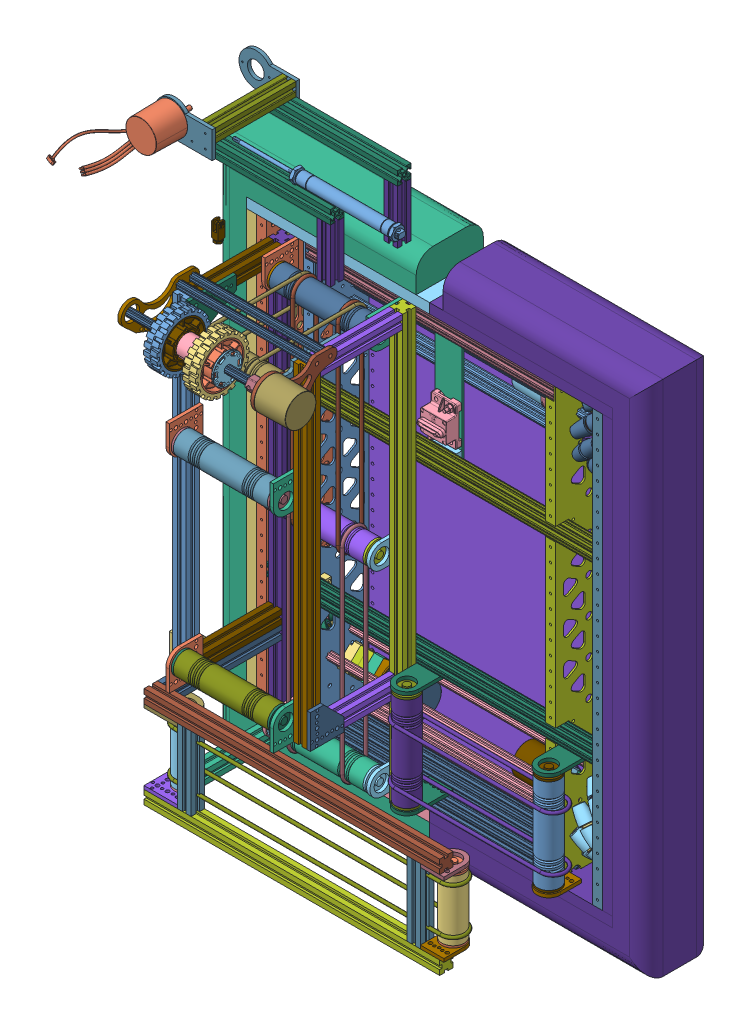
SolidWorks assembly Robot 2020, configuration Default. Lengths in mm. (continued)
Components (placement in the parent): (continued)
- Robot 2020(2)^Robot 2020-1: Robot 2020(2)^Robot 2020 [Default] at origin size (819.15 992.53 549) (virtual) (continued)
  - Fame 2020^Robot 2020(2)_Robot 2020-1: Fame 2020^Robot 2020(2)_Robot 2020 [Default] at origin size (819.15 977.9 171.99) (virtual) (continued)
    - Left Wheel Assembly^Fame 2020_Robot 2020(2)_Robot 2020-1: Left Wheel Assembly^Fame 2020_Robot 2020(2)_Robot 2020 [Default] at (500 0 0) size (65.82 166.11 165.01) (virtual) (continued)
      - 6_Mecanum_Wheel_Left_217-2799^Left Wheel Assembly_Fame 2020_Robot 2020(2)_Robot 2020-1: 6_Mecanum_Wheel_Left_217-2799^Left Wheel Assembly_Fame 2020_Robot 2020(2)_Robot 2020 [Default] x (0 0 1) z (-1 0 0) size (165.01 166.11 65.82) (virtual) (continued)
        - 217-2586-005 Rev2^6_Mecanum_Wheel_Left_217-2799_Left Wheel Assembly_Fame 2020_Robot 2020(2)_Robot 2020-9: 217-2586-005 Rev2^6_Mecanum_Wheel_Left_217-2799_Left Wheel Assembly_Fame 2020_Robot 2020(2)_Robot 2020 [Default] at (85.9856 -351.4028 221.3312) x (-0.32102 -0.630037 -0.707107) z (-0.857032 -0.124484 0.5) size (8.5 8 8) (virtual)
        - 217-2586-005 Rev2^6_Mecanum_Wheel_Left_217-2799_Left Wheel Assembly_Fame 2020_Robot 2020(2)_Robot 2020-10: 217-2586-005 Rev2^6_Mecanum_Wheel_Left_217-2799_Left Wheel Assembly_Fame 2020_Robot 2020(2)_Robot 2020 [Default] at (56.0127 -375.8444 221.3312) x (-0.630037 -0.32102 -0.707107) z (-0.766523 0.403042 0.5) size (8.5 8 8) (virtual)
        - 217-2586-005 Rev2^6_Mecanum_Wheel_Left_217-2799_Left Wheel Assembly_Fame 2020_Robot 2020(2)_Robot 2020-11: 217-2586-005 Rev2^6_Mecanum_Wheel_Left_217-2799_Left Wheel Assembly_Fame 2020_Robot 2020(2)_Robot 2020 [Default] at (17.3977 -378.0003 221.3312) x (-0.698401 0.110616 -0.707107) z (-0.383228 0.776618 0.5) size (8.5 8 8) (virtual)
        - 217-2586-005 Rev2^6_Mecanum_Wheel_Left_217-2799_Left Wheel Assembly_Fame 2020_Robot 2020(2)_Robot 2020-12: 217-2586-005 Rev2^6_Mecanum_Wheel_Left_217-2799_Left Wheel Assembly_Fame 2020_Robot 2020(2)_Robot 2020 [Default] at (-27.1128 -333.4898 233.9884) x (-0.110616 0.698401 -0.707107) z (0.620184 0.60446 0.5) size (8.5 8 8) (virtual)
        - 217-2586-005 Rev2^6_Mecanum_Wheel_Left_217-2799_Left Wheel Assembly_Fame 2020_Robot 2020(2)_Robot 2020-13: 217-2586-005 Rev2^6_Mecanum_Wheel_Left_217-2799_Left Wheel Assembly_Fame 2020_Robot 2020(2)_Robot 2020 [Default] at (-24.9569 -294.8748 233.9884) x (0.32102 0.630037 -0.707107) z (0.857032 0.124484 0.5) size (8.5 8 8) (virtual)
        - 217-2586-005 Rev2^6_Mecanum_Wheel_Left_217-2799_Left Wheel Assembly_Fame 2020_Robot 2020(2)_Robot 2020-14: 217-2586-005 Rev2^6_Mecanum_Wheel_Left_217-2799_Left Wheel Assembly_Fame 2020_Robot 2020(2)_Robot 2020 [Default] at (-0.5153 -264.9019 233.9884) x (0.630037 0.32102 -0.707107) z (0.766523 -0.403042 0.5) size (8.5 8 8) (virtual)
        - 217-2586-005 Rev2^6_Mecanum_Wheel_Left_217-2799_Left Wheel Assembly_Fame 2020_Robot 2020(2)_Robot 2020-15: 217-2586-005 Rev2^6_Mecanum_Wheel_Left_217-2799_Left Wheel Assembly_Fame 2020_Robot 2020(2)_Robot 2020 [Default] at (36.8759 -255.0196 233.9884) x (0.698401 -0.110616 -0.707107) z (0.383228 -0.776618 0.5) size (8.5 8 8) (virtual)
        - 217-2586-005 Rev2^6_Mecanum_Wheel_Left_217-2799_Left Wheel Assembly_Fame 2020_Robot 2020(2)_Robot 2020-16: 217-2586-005 Rev2^6_Mecanum_Wheel_Left_217-2799_Left Wheel Assembly_Fame 2020_Robot 2020(2)_Robot 2020 [Default] at (72.9347 -269.0028 233.9884) x (0.5 -0.5 -0.707107) z (-0.146447 -0.853553 0.5) size (8.5 8 8) (virtual)
        - 217-2586-005 Rev2^6_Mecanum_Wheel_Left_217-2799_Left Wheel Assembly_Fame 2020_Robot 2020(2)_Robot 2020-17: 217-2586-005 Rev2^6_Mecanum_Wheel_Left_217-2799_Left Wheel Assembly_Fame 2020_Robot 2020(2)_Robot 2020 [Default] at (93.8878 -301.5102 233.9884) x (0.110616 -0.698401 -0.707107) z (-0.620184 -0.60446 0.5) size (8.5 8 8) (virtual)
        - 217-2586-005 Rev2^6_Mecanum_Wheel_Left_217-2799_Left Wheel Assembly_Fame 2020_Robot 2020(2)_Robot 2020-18: 217-2586-005 Rev2^6_Mecanum_Wheel_Left_217-2799_Left Wheel Assembly_Fame 2020_Robot 2020(2)_Robot 2020 [Default] at (91.7319 -340.1252 233.9884) x (-0.32102 -0.630037 -0.707107) z (-0.857032 -0.124484 0.5) size (8.5 8 8) (virtual)
        - 217-2586-005 Rev2^6_Mecanum_Wheel_Left_217-2799_Left Wheel Assembly_Fame 2020_Robot 2020(2)_Robot 2020-19: 217-2586-005 Rev2^6_Mecanum_Wheel_Left_217-2799_Left Wheel Assembly_Fame 2020_Robot 2020(2)_Robot 2020 [Default] at (67.2903 -370.0981 233.9884) x (-0.630037 -0.32102 -0.707107) z (-0.766523 0.403042 0.5) size (8.5 8 8) (virtual)
        - 217-2586-005 Rev2^6_Mecanum_Wheel_Left_217-2799_Left Wheel Assembly_Fame 2020_Robot 2020(2)_Robot 2020-20: 217-2586-005 Rev2^6_Mecanum_Wheel_Left_217-2799_Left Wheel Assembly_Fame 2020_Robot 2020(2)_Robot 2020 [Default] at (29.8991 -379.9804 233.9884) x (-0.698401 0.110616 -0.707107) z (-0.383228 0.776618 0.5) size (8.5 8 8) (virtual)
      - 1_2_Hex_Bore_Aluminum_VersaHub_217-2592^Left Wheel Assembly_Fame 2020_Robot 2020(2)_Robot 2020-1: 1_2_Hex_Bore_Aluminum_VersaHub_217-2592^Left Wheel Assembly_Fame 2020_Robot 2020(2)_Robot 2020 [Default] at (-239.7248 -317.5 33.3875) x (-1 0 0) z (0 0.707107 0.707107) size (12.7 55.88 55.88) (virtual)
    - NEO Gearbox 2-stage Custom v5(Mirror) (2)^Fame 2020_Robot 2020(2)_Robot 2020-1: NEO Gearbox 2-stage Custom v5(Mirror) (2)^Fame 2020_Robot 2020(2)_Robot 2020 [Default] at (0 0 425) x (1 0 0) z (0 0 -1) size (164.9 90.53 90.53) (virtual)
      - VersaPlanetary_4_1_Gear_Kit_217-2818 v1(Mirror) (2)^NEO Gearbox 2-stage Custom v5(Mirror) (2)_Fame 2020_Robot 2020(2)_Robot 2020-1: VersaPlanetary_4_1_Gear_Kit_217-2818 v1(Mirror) (2)^NEO Gearbox 2-stage Custom v5(Mirror) (2)_Fame 2020_Robot 2020(2)_Robot 2020 [Default] at (-15.25 22.225 0) x (0 -0.707107 -0.707107) z (1 0 0) size (35.49 35.49 17.4) (virtual)
        - 217-2725-001 Rev1_24t Sun(Mirror) (2)^VersaPlanetary_4_1_Gear_Kit_217-2818 v1(Mirror) (2)_NEO Gearbox 2-stage Custom v5(Mirror) (2)_Fame 2020_Robot 2020(2)_Robot 2020-1: 217-2725-001 Rev1_24t Sun(Mirror) (2)^VersaPlanetary_4_1_Gear_Kit_217-2818 v1(Mirror) (2)_NEO Gearbox 2-stage Custom v5(Mirror) (2)_Fame 2020_Robot 2020(2)_Robot 2020 [Default] at (-36.69 -517.1337 209.675) x (0.707107 0.707107 0) z (0 0 1) size (14.4 14.45 12.7) (virtual)
        - 217-2725-002 Rev1_24t Planet(Mirror) (2)^VersaPlanetary_4_1_Gear_Kit_217-2818 v1(Mirror) (2)_NEO Gearbox 2-stage Custom v5(Mirror) (2)_Fame 2020_Robot 2020(2)_Robot 2020-1: 217-2725-002 Rev1_24t Planet(Mirror) (2)^VersaPlanetary_4_1_Gear_Kit_217-2818 v1(Mirror) (2)_NEO Gearbox 2-stage Custom v5(Mirror) (2)_Fame 2020_Robot 2020(2)_Robot 2020 [Default] at (-45.2382 -525.6819 212.025) x (-0.793353 0.608761 0) z (0 0 -1) size (13.12 13.1 8) (virtual)
        - 217-2725-002 Rev1_24t Planet(Mirror) (2)^VersaPlanetary_4_1_Gear_Kit_217-2818 v1(Mirror) (2)_NEO Gearbox 2-stage Custom v5(Mirror) (2)_Fame 2020_Robot 2020(2)_Robot 2020-2: 217-2725-002 Rev1_24t Planet(Mirror) (2)^VersaPlanetary_4_1_Gear_Kit_217-2818 v1(Mirror) (2)_NEO Gearbox 2-stage Custom v5(Mirror) (2)_Fame 2020_Robot 2020(2)_Robot 2020 [Default] at (-28.1418 -525.6819 212.025) x (-0.608761 -0.793353 0) z (0 0 -1) size (13.12 13.1 8) (virtual)
        - 217-2725-002 Rev1_24t Planet(Mirror) (2)^VersaPlanetary_4_1_Gear_Kit_217-2818 v1(Mirror) (2)_NEO Gearbox 2-stage Custom v5(Mirror) (2)_Fame 2020_Robot 2020(2)_Robot 2020-3: 217-2725-002 Rev1_24t Planet(Mirror) (2)^VersaPlanetary_4_1_Gear_Kit_217-2818 v1(Mirror) (2)_NEO Gearbox 2-stage Custom v5(Mirror) (2)_Fame 2020_Robot 2020(2)_Robot 2020 [Default] at (-28.1418 -508.5855 212.025) x (0.793353 -0.608761 0) z (0 0 -1) size (13.12 13.1 8) (virtual)
        - 217-2725-002 Rev1_24t Planet(Mirror) (2)^VersaPlanetary_4_1_Gear_Kit_217-2818 v1(Mirror) (2)_NEO Gearbox 2-stage Custom v5(Mirror) (2)_Fame 2020_Robot 2020(2)_Robot 2020-4: 217-2725-002 Rev1_24t Planet(Mirror) (2)^VersaPlanetary_4_1_Gear_Kit_217-2818 v1(Mirror) (2)_NEO Gearbox 2-stage Custom v5(Mirror) (2)_Fame 2020_Robot 2020(2)_Robot 2020 [Default] at (-45.2382 -508.5855 212.025) x (0.608761 0.793353 0) z (0 0 -1) size (13.12 13.1 8) (virtual)
        - 217-2724-002 Rev1(Mirror) (2)^VersaPlanetary_4_1_Gear_Kit_217-2818 v1(Mirror) (2)_NEO Gearbox 2-stage Custom v5(Mirror) (2)_Fame 2020_Robot 2020(2)_Robot 2020-1: 217-2724-002 Rev1(Mirror) (2)^VersaPlanetary_4_1_Gear_Kit_217-2818 v1(Mirror) (2)_NEO Gearbox 2-stage Custom v5(Mirror) (2)_Fame 2020_Robot 2020(2)_Robot 2020 [Default] at (-36.69 -517.1337 218.375) x (1 0 0) z (0 0 -1) size (34.7 34.7 4.7) (virtual)
        - 217-2625-010 Rev1(Mirror) (2)^VersaPlanetary_4_1_Gear_Kit_217-2818 v1(Mirror) (2)_NEO Gearbox 2-stage Custom v5(Mirror) (2)_Fame 2020_Robot 2020(2)_Robot 2020-1: 217-2625-010 Rev1(Mirror) (2)^VersaPlanetary_4_1_Gear_Kit_217-2818 v1(Mirror) (2)_NEO Gearbox 2-stage Custom v5(Mirror) (2)_Fame 2020_Robot 2020(2)_Robot 2020 [Default] at (-45.2382 -525.6819 214.725) x (0.854322 0.519745 0) z (0 0 1) size (4 4 12) (virtual)
        - 217-2625-010 Rev1(Mirror) (2)^VersaPlanetary_4_1_Gear_Kit_217-2818 v1(Mirror) (2)_NEO Gearbox 2-stage Custom v5(Mirror) (2)_Fame 2020_Robot 2020(2)_Robot 2020-2: 217-2625-010 Rev1(Mirror) (2)^VersaPlanetary_4_1_Gear_Kit_217-2818 v1(Mirror) (2)_NEO Gearbox 2-stage Custom v5(Mirror) (2)_Fame 2020_Robot 2020(2)_Robot 2020 [Default] at (-28.1418 -525.6819 214.725) x (-0.519745 0.854322 0) z (0 0 1) size (4 4 12) (virtual)
        - 217-2625-010 Rev1(Mirror) (2)^VersaPlanetary_4_1_Gear_Kit_217-2818 v1(Mirror) (2)_NEO Gearbox 2-stage Custom v5(Mirror) (2)_Fame 2020_Robot 2020(2)_Robot 2020-3: 217-2625-010 Rev1(Mirror) (2)^VersaPlanetary_4_1_Gear_Kit_217-2818 v1(Mirror) (2)_NEO Gearbox 2-stage Custom v5(Mirror) (2)_Fame 2020_Robot 2020(2)_Robot 2020 [Default] at (-28.1418 -508.5855 214.725) x (-0.854322 -0.519745 0) z (0 0 1) size (4 4 12) (virtual)
        - 217-2625-010 Rev1(Mirror) (2)^VersaPlanetary_4_1_Gear_Kit_217-2818 v1(Mirror) (2)_NEO Gearbox 2-stage Custom v5(Mirror) (2)_Fame 2020_Robot 2020(2)_Robot 2020-4: 217-2625-010 Rev1(Mirror) (2)^VersaPlanetary_4_1_Gear_Kit_217-2818 v1(Mirror) (2)_NEO Gearbox 2-stage Custom v5(Mirror) (2)_Fame 2020_Robot 2020(2)_Robot 2020 [Default] at (-45.2382 -508.5855 214.725) x (0.519745 -0.854322 0) z (0 0 1) size (4 4 12) (virtual)
      - 217-2625-026 Rev1(Mirror) (2)^NEO Gearbox 2-stage Custom v5(Mirror) (2)_Fame 2020_Robot 2020(2)_Robot 2020-1: 217-2625-026 Rev1(Mirror) (2)^NEO Gearbox 2-stage Custom v5(Mirror) (2)_Fame 2020_Robot 2020(2)_Robot 2020 [Default] at (211.875 -317.5 391.6125) x (0 -0.707107 -0.707107) z (1 0 0) size (44.45 42 18.12) (virtual)
      - 217-2742-001 Rev4(Mirror) (2)^NEO Gearbox 2-stage Custom v5(Mirror) (2)_Fame 2020_Robot 2020(2)_Robot 2020-1: 217-2742-001 Rev4(Mirror) (2)^NEO Gearbox 2-stage Custom v5(Mirror) (2)_Fame 2020_Robot 2020(2)_Robot 2020 [Default] at (218.5752 -317.5 391.6125) x (1 0 0) z (0 -0.63857 0.769564) size (7 28 28) (virtual)
      - 217-2742-001 Rev4(Mirror) (2)^NEO Gearbox 2-stage Custom v5(Mirror) (2)_Fame 2020_Robot 2020(2)_Robot 2020-2: 217-2742-001 Rev4(Mirror) (2)^NEO Gearbox 2-stage Custom v5(Mirror) (2)_Fame 2020_Robot 2020(2)_Robot 2020 [Default] at (226.5752 -317.5 391.6125) x (1 0 0) z (0 -0.707107 0.707107) size (7 28 28) (virtual)
      - 217-2625-017 Rev1_9714K61(Mirror) (2)^NEO Gearbox 2-stage Custom v5(Mirror) (2)_Fame 2020_Robot 2020(2)_Robot 2020-1: 217-2625-017 Rev1_9714K61(Mirror) (2)^NEO Gearbox 2-stage Custom v5(Mirror) (2)_Fame 2020_Robot 2020(2)_Robot 2020 [Default] at (225.795 -317.6887 391.9075) x (0 0.983393 -0.181491) z (0 0.181491 0.983393) size (28.51 4.98 27.43) (virtual)
      - 217-2625-025 Rev1(Mirror) (2)^NEO Gearbox 2-stage Custom v5(Mirror) (2)_Fame 2020_Robot 2020(2)_Robot 2020-1: 217-2625-025 Rev1(Mirror) (2)^NEO Gearbox 2-stage Custom v5(Mirror) (2)_Fame 2020_Robot 2020(2)_Robot 2020 [Default] at (182.475 -317.5 391.6125) x (0 -0.707107 -0.707107) z (1 0 0) size (44.45 42 18) (virtual)
      - 217-2816-001 Rev1(Mirror) (2)^NEO Gearbox 2-stage Custom v5(Mirror) (2)_Fame 2020_Robot 2020(2)_Robot 2020-1: 217-2816-001 Rev1(Mirror) (2)^NEO Gearbox 2-stage Custom v5(Mirror) (2)_Fame 2020_Robot 2020(2)_Robot 2020 [Default] at (212.025 -317.5 391.6125) x (0 -0.707107 -0.707107) z (-1 0 0) size (42 42 14.5) (virtual)
      - 217-2816-001 Rev1(Mirror) (2)^NEO Gearbox 2-stage Custom v5(Mirror) (2)_Fame 2020_Robot 2020(2)_Robot 2020-2: 217-2816-001 Rev1(Mirror) (2)^NEO Gearbox 2-stage Custom v5(Mirror) (2)_Fame 2020_Robot 2020(2)_Robot 2020 [Default] at (199.325 -317.5 391.6125) x (0 -0.707107 -0.707107) z (-1 0 0) size (42 42 14.5) (virtual)
      - 217-4649-001 Rev1(Mirror) (2)^NEO Gearbox 2-stage Custom v5(Mirror) (2)_Fame 2020_Robot 2020(2)_Robot 2020-1: 217-4649-001 Rev1(Mirror) (2)^NEO Gearbox 2-stage Custom v5(Mirror) (2)_Fame 2020_Robot 2020(2)_Robot 2020 [Default] at (185.629 -317.5 391.6125) x (0 -0.707107 -0.707107) z (-1 0 0) size (18 18 13) (virtual)
      - VersaPlanetary_CIM_Adapter_217-4018 v1(Mirror) (2)^NEO Gearbox 2-stage Custom v5(Mirror) (2)_Fame 2020_Robot 2020(2)_Robot 2020-1: VersaPlanetary_CIM_Adapter_217-4018 v1(Mirror) (2)^NEO Gearbox 2-stage Custom v5(Mirror) (2)_Fame 2020_Robot 2020(2)_Robot 2020 [Default] at (165.15 -317.5 391.6125) x (0 -0.707107 -0.707107) z (0 -0.707107 0.707107) size (64.01 21.55 64.01) (virtual)
      - NEO Motor REV-21-1650 v2(Mirror) (2)^NEO Gearbox 2-stage Custom v5(Mirror) (2)_Fame 2020_Robot 2020(2)_Robot 2020-1: NEO Motor REV-21-1650 v2(Mirror) (2)^NEO Gearbox 2-stage Custom v5(Mirror) (2)_Fame 2020_Robot 2020(2)_Robot 2020 [Default] at (153.625 -317.5 391.6125) x (0 -0.707107 0.707107) z (-1 0 0) size (61.14 61.02 93.25) (virtual)
      - 3_1 Output Shaft Custom v6(Mirror) (2)^NEO Gearbox 2-stage Custom v5(Mirror) (2)_Fame 2020_Robot 2020(2)_Robot 2020-1: 3_1 Output Shaft Custom v6(Mirror) (2)^NEO Gearbox 2-stage Custom v5(Mirror) (2)_Fame 2020_Robot 2020(2)_Robot 2020 [Default] at (211.3752 -317.5 391.6125) x (1 0 0) z (0 -0.707107 0.707107) size (48.9 34.7 34.7) (virtual)
    - Left Wheel Assembly v4(Mirror) (2)^Fame 2020_Robot 2020(2)_Robot 2020-1: Left Wheel Assembly v4(Mirror) (2)^Fame 2020_Robot 2020(2)_Robot 2020 [Default] at (500 0 0) x (1 0 0) z (0 0 -1) size (65.82 166.11 165.01) (virtual)
      - 6_Mecanum_Wheel_Left_217-2799 v1(Mirror) (2)^Left Wheel Assembly v4(Mirror) (2)_Fame 2020_Robot 2020(2)_Robot 2020-1: 6_Mecanum_Wheel_Left_217-2799 v1(Mirror) (2)^Left Wheel Assembly v4(Mirror) (2)_Fame 2020_Robot 2020(2)_Robot 2020 [Default] x (0 0 -1) z (1 0 0) size (165.01 166.11 65.82) (virtual)
        - 217-2799-001 Rev1(Mirror) (2)^6_Mecanum_Wheel_Left_217-2799 v1(Mirror) (2)_Left Wheel Assembly v4(Mirror) (2)_Fame 2020_Robot 2020(2)_Robot 2020-1: 217-2799-001 Rev1(Mirror) (2)^6_Mecanum_Wheel_Left_217-2799 v1(Mirror) (2)_Left Wheel Assembly v4(Mirror) (2)_Fame 2020_Robot 2020(2)_Robot 2020 [Default] at (33.3875 -317.5 -234.0098) x (0.707107 0.707107 0) z (0 0 1) size (95.78 100.46 28.55) (virtual)
        - 217-2799-001 Rev1(Mirror) (2)^6_Mecanum_Wheel_Left_217-2799 v1(Mirror) (2)_Left Wheel Assembly v4(Mirror) (2)_Fame 2020_Robot 2020(2)_Robot 2020-2: 217-2799-001 Rev1(Mirror) (2)^6_Mecanum_Wheel_Left_217-2799 v1(Mirror) (2)_Left Wheel Assembly v4(Mirror) (2)_Fame 2020_Robot 2020(2)_Robot 2020 [Default] at (33.3875 -317.5 -221.3098) x (-0.987688 -0.156434 0) z (0 0 -1) size (95.78 100.46 28.55) (virtual)
        - 217-2799-002 Rev1(Mirror) (2)^6_Mecanum_Wheel_Left_217-2799 v1(Mirror) (2)_Left Wheel Assembly v4(Mirror) (2)_Fame 2020_Robot 2020(2)_Robot 2020-1: 217-2799-002 Rev1(Mirror) (2)^6_Mecanum_Wheel_Left_217-2799 v1(Mirror) (2)_Left Wheel Assembly v4(Mirror) (2)_Fame 2020_Robot 2020(2)_Robot 2020 [Default] at (4.057 -346.8305 -227.6598) x (-0.707107 0.707107 0) z (0.707107 0.707107 0) size (26.84 25.39 30.1) (virtual)
        - 217-2799-002 Rev1(Mirror) (2)^6_Mecanum_Wheel_Left_217-2799 v1(Mirror) (2)_Left Wheel Assembly v4(Mirror) (2)_Fame 2020_Robot 2020(2)_Robot 2020-2: 217-2799-002 Rev1(Mirror) (2)^6_Mecanum_Wheel_Left_217-2799 v1(Mirror) (2)_Left Wheel Assembly v4(Mirror) (2)_Fame 2020_Robot 2020(2)_Robot 2020 [Default] at (-7.5815 -323.9888 -227.6598) x (-0.156434 0.987688 0) z (0.987688 0.156434 0) size (26.84 25.39 30.1) (virtual)
        - 217-2799-002 Rev1(Mirror) (2)^6_Mecanum_Wheel_Left_217-2799 v1(Mirror) (2)_Left Wheel Assembly v4(Mirror) (2)_Fame 2020_Robot 2020(2)_Robot 2020-3: 217-2799-002 Rev1(Mirror) (2)^6_Mecanum_Wheel_Left_217-2799 v1(Mirror) (2)_Left Wheel Assembly v4(Mirror) (2)_Fame 2020_Robot 2020(2)_Robot 2020 [Default] at (-3.5711 -298.6686 -227.6598) x (0.45399 0.891007 0) z (0.891007 -0.45399 0) size (26.84 25.39 30.1) (virtual)
        - 217-2799-002 Rev1(Mirror) (2)^6_Mecanum_Wheel_Left_217-2799 v1(Mirror) (2)_Left Wheel Assembly v4(Mirror) (2)_Fame 2020_Robot 2020(2)_Robot 2020-4: 217-2799-002 Rev1(Mirror) (2)^6_Mecanum_Wheel_Left_217-2799 v1(Mirror) (2)_Left Wheel Assembly v4(Mirror) (2)_Fame 2020_Robot 2020(2)_Robot 2020 [Default] at (14.5561 -280.5414 -227.6598) x (0.891007 0.45399 0) z (0.45399 -0.891007 0) size (26.84 25.39 30.1) (virtual)
        - 217-2799-002 Rev1(Mirror) (2)^6_Mecanum_Wheel_Left_217-2799 v1(Mirror) (2)_Left Wheel Assembly v4(Mirror) (2)_Fame 2020_Robot 2020(2)_Robot 2020-5: 217-2799-002 Rev1(Mirror) (2)^6_Mecanum_Wheel_Left_217-2799 v1(Mirror) (2)_Left Wheel Assembly v4(Mirror) (2)_Fame 2020_Robot 2020(2)_Robot 2020 [Default] at (39.8763 -276.531 -227.6598) x (0.987688 -0.156434 0) z (-0.156434 -0.987688 0) size (26.84 25.39 30.1) (virtual)
        - 217-2799-002 Rev1(Mirror) (2)^6_Mecanum_Wheel_Left_217-2799 v1(Mirror) (2)_Left Wheel Assembly v4(Mirror) (2)_Fame 2020_Robot 2020(2)_Robot 2020-6: 217-2799-002 Rev1(Mirror) (2)^6_Mecanum_Wheel_Left_217-2799 v1(Mirror) (2)_Left Wheel Assembly v4(Mirror) (2)_Fame 2020_Robot 2020(2)_Robot 2020 [Default] at (62.718 -288.1695 -227.6598) x (0.707107 -0.707107 0) z (-0.707107 -0.707107 0) size (26.84 25.39 30.1) (virtual)
        - 217-2799-002 Rev1(Mirror) (2)^6_Mecanum_Wheel_Left_217-2799 v1(Mirror) (2)_Left Wheel Assembly v4(Mirror) (2)_Fame 2020_Robot 2020(2)_Robot 2020-7: 217-2799-002 Rev1(Mirror) (2)^6_Mecanum_Wheel_Left_217-2799 v1(Mirror) (2)_Left Wheel Assembly v4(Mirror) (2)_Fame 2020_Robot 2020(2)_Robot 2020 [Default] at (74.3565 -311.0112 -227.6598) x (0.156434 -0.987688 0) z (-0.987688 -0.156434 0) size (26.84 25.39 30.1) (virtual)
        - 217-2799-002 Rev1(Mirror) (2)^6_Mecanum_Wheel_Left_217-2799 v1(Mirror) (2)_Left Wheel Assembly v4(Mirror) (2)_Fame 2020_Robot 2020(2)_Robot 2020-8: 217-2799-002 Rev1(Mirror) (2)^6_Mecanum_Wheel_Left_217-2799 v1(Mirror) (2)_Left Wheel Assembly v4(Mirror) (2)_Fame 2020_Robot 2020(2)_Robot 2020 [Default] at (70.3461 -336.3314 -227.6598) x (-0.45399 -0.891007 0) z (-0.891007 0.45399 0) size (26.84 25.39 30.1) (virtual)
        - 217-2799-002 Rev1(Mirror) (2)^6_Mecanum_Wheel_Left_217-2799 v1(Mirror) (2)_Left Wheel Assembly v4(Mirror) (2)_Fame 2020_Robot 2020(2)_Robot 2020-9: 217-2799-002 Rev1(Mirror) (2)^6_Mecanum_Wheel_Left_217-2799 v1(Mirror) (2)_Left Wheel Assembly v4(Mirror) (2)_Fame 2020_Robot 2020(2)_Robot 2020 [Default] at (52.2189 -354.4586 -227.6598) x (-0.891007 -0.45399 0) z (-0.45399 0.891007 0) size (26.84 25.39 30.1) (virtual)
        - 217-2799-002 Rev1(Mirror) (2)^6_Mecanum_Wheel_Left_217-2799 v1(Mirror) (2)_Left Wheel Assembly v4(Mirror) (2)_Fame 2020_Robot 2020(2)_Robot 2020-10: 217-2799-002 Rev1(Mirror) (2)^6_Mecanum_Wheel_Left_217-2799 v1(Mirror) (2)_Left Wheel Assembly v4(Mirror) (2)_Fame 2020_Robot 2020(2)_Robot 2020 [Default] at (26.8987 -358.469 -227.6598) x (-0.987688 0.156434 0) z (0.156434 0.987688 0) size (26.84 25.39 30.1) (virtual)
        - 217-2586-003 Rev2(Mirror) (2)^6_Mecanum_Wheel_Left_217-2799 v1(Mirror) (2)_Left Wheel Assembly v4(Mirror) (2)_Fame 2020_Robot 2020(2)_Robot 2020-1: 217-2586-003 Rev2(Mirror) (2)^6_Mecanum_Wheel_Left_217-2799 v1(Mirror) (2)_Left Wheel Assembly v4(Mirror) (2)_Fame 2020_Robot 2020(2)_Robot 2020 [Default] at (-13.4676 -358.6894 -223.6536) x (0.41944 0.854155 -0.30739) z (0.757674 -0.142894 0.636798) size (19.46 28.57 19.46) (virtual)
        - 217-2586-003 Rev2(Mirror) (2)^6_Mecanum_Wheel_Left_217-2799 v1(Mirror) (2)_Left Wheel Assembly v4(Mirror) (2)_Fame 2020_Robot 2020(2)_Robot 2020-2: 217-2586-003 Rev2(Mirror) (2)^6_Mecanum_Wheel_Left_217-2799 v1(Mirror) (2)_Left Wheel Assembly v4(Mirror) (2)_Fame 2020_Robot 2020(2)_Robot 2020 [Default] at (-7.8019 -364.3551 -231.666) x (0.847342 0.451134 0.280161) z (-0.17892 0.739241 -0.649238) size (19.46 28.57 19.46) (virtual)
        - 217-2586-003 Rev2(Mirror) (2)^6_Mecanum_Wheel_Left_217-2799 v1(Mirror) (2)_Left Wheel Assembly v4(Mirror) (2)_Fame 2020_Robot 2020(2)_Robot 2020-3: 217-2586-003 Rev2(Mirror) (2)^6_Mecanum_Wheel_Left_217-2799 v1(Mirror) (2)_Left Wheel Assembly v4(Mirror) (2)_Fame 2020_Robot 2020(2)_Robot 2020 [Default] at (-27.4761 -331.196 -231.666) x (0.950684 -0.13308 0.280161) z (0.289766 0.703225 -0.649238) size (19.46 28.57 19.46) (virtual)
        - 217-2586-003 Rev2(Mirror) (2)^6_Mecanum_Wheel_Left_217-2799 v1(Mirror) (2)_Left Wheel Assembly v4(Mirror) (2)_Fame 2020_Robot 2020(2)_Robot 2020-4: 217-2586-003 Rev2(Mirror) (2)^6_Mecanum_Wheel_Left_217-2799 v1(Mirror) (2)_Left Wheel Assembly v4(Mirror) (2)_Fame 2020_Robot 2020(2)_Robot 2020 [Default] at (-23.9025 -292.8056 -231.666) x (0.690897 -0.666462 0.280161) z (0.647771 0.398601 -0.649238) size (19.46 28.57 19.46) (virtual)
        - 217-2586-003 Rev2(Mirror) (2)^6_Mecanum_Wheel_Left_217-2799 v1(Mirror) (2)_Left Wheel Assembly v4(Mirror) (2)_Fame 2020_Robot 2020(2)_Robot 2020-5: 217-2586-003 Rev2(Mirror) (2)^6_Mecanum_Wheel_Left_217-2799 v1(Mirror) (2)_Left Wheel Assembly v4(Mirror) (2)_Fame 2020_Robot 2020(2)_Robot 2020 [Default] at (1.5539 -263.8475 -231.666) x (0.167211 -0.945278 0.280161) z (0.75835 -0.058276 -0.649238) size (19.46 28.57 19.46) (virtual)
        - 217-2586-003 Rev2(Mirror) (2)^6_Mecanum_Wheel_Left_217-2799 v1(Mirror) (2)_Left Wheel Assembly v4(Mirror) (2)_Fame 2020_Robot 2020(2)_Robot 2020-6: 217-2586-003 Rev2(Mirror) (2)^6_Mecanum_Wheel_Left_217-2799 v1(Mirror) (2)_Left Wheel Assembly v4(Mirror) (2)_Fame 2020_Robot 2020(2)_Robot 2020 [Default] at (39.1697 -255.3829 -231.666) x (-0.420344 -0.86303 0.280161) z (0.579264 -0.492893 -0.649238) size (19.46 28.57 19.46) (virtual)
        - 217-2586-003 Rev2(Mirror) (2)^6_Mecanum_Wheel_Left_217-2799 v1(Mirror) (2)_Left Wheel Assembly v4(Mirror) (2)_Fame 2020_Robot 2020(2)_Robot 2020-7: 217-2586-003 Rev2(Mirror) (2)^6_Mecanum_Wheel_Left_217-2799 v1(Mirror) (2)_Left Wheel Assembly v4(Mirror) (2)_Fame 2020_Robot 2020(2)_Robot 2020 [Default] at (74.5769 -270.6449 -231.666) x (-0.847342 -0.451134 0.280161) z (0.17892 -0.739241 -0.649238) size (19.46 28.57 19.46) (virtual)
        - 217-2586-003 Rev2(Mirror) (2)^6_Mecanum_Wheel_Left_217-2799 v1(Mirror) (2)_Left Wheel Assembly v4(Mirror) (2)_Fame 2020_Robot 2020(2)_Robot 2020-8: 217-2586-003 Rev2(Mirror) (2)^6_Mecanum_Wheel_Left_217-2799 v1(Mirror) (2)_Left Wheel Assembly v4(Mirror) (2)_Fame 2020_Robot 2020(2)_Robot 2020 [Default] at (94.2511 -303.804 -231.666) x (-0.950684 0.13308 0.280161) z (-0.289766 -0.703225 -0.649238) size (19.46 28.57 19.46) (virtual)
        - 217-2586-003 Rev2(Mirror) (2)^6_Mecanum_Wheel_Left_217-2799 v1(Mirror) (2)_Left Wheel Assembly v4(Mirror) (2)_Fame 2020_Robot 2020(2)_Robot 2020-9: 217-2586-003 Rev2(Mirror) (2)^6_Mecanum_Wheel_Left_217-2799 v1(Mirror) (2)_Left Wheel Assembly v4(Mirror) (2)_Fame 2020_Robot 2020(2)_Robot 2020 [Default] at (90.6775 -342.1944 -231.666) x (-0.690897 0.666462 0.280161) z (-0.647771 -0.398601 -0.649238) size (19.46 28.57 19.46) (virtual)
        - 217-2586-003 Rev2(Mirror) (2)^6_Mecanum_Wheel_Left_217-2799 v1(Mirror) (2)_Left Wheel Assembly v4(Mirror) (2)_Fame 2020_Robot 2020(2)_Robot 2020-10: 217-2586-003 Rev2(Mirror) (2)^6_Mecanum_Wheel_Left_217-2799 v1(Mirror) (2)_Left Wheel Assembly v4(Mirror) (2)_Fame 2020_Robot 2020(2)_Robot 2020 [Default] at (65.2211 -371.1525 -231.666) x (-0.167211 0.945278 0.280161) z (-0.75835 0.058276 -0.649238) size (19.46 28.57 19.46) (virtual)
        - 217-2586-003 Rev2(Mirror) (2)^6_Mecanum_Wheel_Left_217-2799 v1(Mirror) (2)_Left Wheel Assembly v4(Mirror) (2)_Fame 2020_Robot 2020(2)_Robot 2020-11: 217-2586-003 Rev2(Mirror) (2)^6_Mecanum_Wheel_Left_217-2799 v1(Mirror) (2)_Left Wheel Assembly v4(Mirror) (2)_Fame 2020_Robot 2020(2)_Robot 2020 [Default] at (27.6053 -379.6171 -231.666) x (0.420344 0.86303 0.280161) z (-0.579264 0.492893 -0.649238) size (19.46 28.57 19.46) (virtual)
        - 217-2586-003 Rev2(Mirror) (2)^6_Mecanum_Wheel_Left_217-2799 v1(Mirror) (2)_Left Wheel Assembly v4(Mirror) (2)_Fame 2020_Robot 2020(2)_Robot 2020-12: 217-2586-003 Rev2(Mirror) (2)^6_Mecanum_Wheel_Left_217-2799 v1(Mirror) (2)_Left Wheel Assembly v4(Mirror) (2)_Fame 2020_Robot 2020(2)_Robot 2020 [Default] at (-28.7296 -323.2822 -223.6536) x (0.841394 0.444485 -0.30739) z (0.52898 -0.560953 0.636798) size (19.46 28.57 19.46) (virtual)
        - 217-2586-003 Rev2(Mirror) (2)^6_Mecanum_Wheel_Left_217-2799 v1(Mirror) (2)_Left Wheel Assembly v4(Mirror) (2)_Fame 2020_Robot 2020(2)_Robot 2020-13: 217-2586-003 Rev2(Mirror) (2)^6_Mecanum_Wheel_Left_217-2799 v1(Mirror) (2)_Left Wheel Assembly v4(Mirror) (2)_Fame 2020_Robot 2020(2)_Robot 2020 [Default] at (-20.265 -285.6664 -223.6536) x (0.941964 -0.134963 -0.30739) z (0.098234 -0.764747 0.636798) size (19.46 28.57 19.46) (virtual)
        - 217-2586-003 Rev2(Mirror) (2)^6_Mecanum_Wheel_Left_217-2799 v1(Mirror) (2)_Left Wheel Assembly v4(Mirror) (2)_Fame 2020_Robot 2020(2)_Robot 2020-14: 217-2586-003 Rev2(Mirror) (2)^6_Mecanum_Wheel_Left_217-2799 v1(Mirror) (2)_Left Wheel Assembly v4(Mirror) (2)_Fame 2020_Robot 2020(2)_Robot 2020 [Default] at (8.6931 -260.21 -223.6536) x (0.682736 -0.66286 -0.30739) z (-0.370035 -0.676434 0.636798) size (19.46 28.57 19.46) (virtual)
        - 217-2586-003 Rev2(Mirror) (2)^6_Mecanum_Wheel_Left_217-2799 v1(Mirror) (2)_Left Wheel Assembly v4(Mirror) (2)_Fame 2020_Robot 2020(2)_Robot 2020-15: 217-2586-003 Rev2(Mirror) (2)^6_Mecanum_Wheel_Left_217-2799 v1(Mirror) (2)_Left Wheel Assembly v4(Mirror) (2)_Fame 2020_Robot 2020(2)_Robot 2020 [Default] at (47.0835 -256.6364 -223.6536) x (0.162726 -0.937567 -0.30739) z (-0.696962 -0.329746 0.636798) size (19.46 28.57 19.46) (virtual)
        - 217-2586-003 Rev2(Mirror) (2)^6_Mecanum_Wheel_Left_217-2799 v1(Mirror) (2)_Left Wheel Assembly v4(Mirror) (2)_Fame 2020_Robot 2020(2)_Robot 2020-16: 217-2586-003 Rev2(Mirror) (2)^6_Mecanum_Wheel_Left_217-2799 v1(Mirror) (2)_Left Wheel Assembly v4(Mirror) (2)_Fame 2020_Robot 2020(2)_Robot 2020 [Default] at (80.2426 -276.3106 -223.6536) x (-0.41944 -0.854155 -0.30739) z (-0.757674 0.142894 0.636798) size (19.46 28.57 19.46) (virtual)
        - 217-2586-003 Rev2(Mirror) (2)^6_Mecanum_Wheel_Left_217-2799 v1(Mirror) (2)_Left Wheel Assembly v4(Mirror) (2)_Fame 2020_Robot 2020(2)_Robot 2020-17: 217-2586-003 Rev2(Mirror) (2)^6_Mecanum_Wheel_Left_217-2799 v1(Mirror) (2)_Left Wheel Assembly v4(Mirror) (2)_Fame 2020_Robot 2020(2)_Robot 2020 [Default] at (95.5046 -311.7178 -223.6536) x (-0.841394 -0.444485 -0.30739) z (-0.52898 0.560953 0.636798) size (19.46 28.57 19.46) (virtual)
        - 217-2586-003 Rev2(Mirror) (2)^6_Mecanum_Wheel_Left_217-2799 v1(Mirror) (2)_Left Wheel Assembly v4(Mirror) (2)_Fame 2020_Robot 2020(2)_Robot 2020-18: 217-2586-003 Rev2(Mirror) (2)^6_Mecanum_Wheel_Left_217-2799 v1(Mirror) (2)_Left Wheel Assembly v4(Mirror) (2)_Fame 2020_Robot 2020(2)_Robot 2020 [Default] at (87.04 -349.3336 -223.6536) x (-0.941964 0.134963 -0.30739) z (-0.098234 0.764747 0.636798) size (19.46 28.57 19.46) (virtual)
        - 217-2586-003 Rev2(Mirror) (2)^6_Mecanum_Wheel_Left_217-2799 v1(Mirror) (2)_Left Wheel Assembly v4(Mirror) (2)_Fame 2020_Robot 2020(2)_Robot 2020-19: 217-2586-003 Rev2(Mirror) (2)^6_Mecanum_Wheel_Left_217-2799 v1(Mirror) (2)_Left Wheel Assembly v4(Mirror) (2)_Fame 2020_Robot 2020(2)_Robot 2020 [Default] at (58.0819 -374.79 -223.6536) x (-0.682736 0.66286 -0.30739) z (0.370035 0.676434 0.636798) size (19.46 28.57 19.46) (virtual)
        - 217-2586-003 Rev2(Mirror) (2)^6_Mecanum_Wheel_Left_217-2799 v1(Mirror) (2)_Left Wheel Assembly v4(Mirror) (2)_Fame 2020_Robot 2020(2)_Robot 2020-20: 217-2586-003 Rev2(Mirror) (2)^6_Mecanum_Wheel_Left_217-2799 v1(Mirror) (2)_Left Wheel Assembly v4(Mirror) (2)_Fame 2020_Robot 2020(2)_Robot 2020 [Default] at (19.6915 -378.3636 -223.6536) x (-0.162726 0.937567 -0.30739) z (0.696962 0.329746 0.636798) size (19.46 28.57 19.46) (virtual)
        - 217-2586-004 Rev1(Mirror) (2)^6_Mecanum_Wheel_Left_217-2799 v1(Mirror) (2)_Left Wheel Assembly v4(Mirror) (2)_Fame 2020_Robot 2020(2)_Robot 2020-1: 217-2586-004 Rev1(Mirror) (2)^6_Mecanum_Wheel_Left_217-2799 v1(Mirror) (2)_Left Wheel Assembly v4(Mirror) (2)_Fame 2020_Robot 2020(2)_Robot 2020 [Default] at (-10.3479 -361.809 -228.0654) x (-0.690521 -0.722949 0.02293) z (-0.522667 0.476807 -0.706735) size (25.9 28.58 25.9) (virtual)
        - 217-2586-004 Rev1(Mirror) (2)^6_Mecanum_Wheel_Left_217-2799 v1(Mirror) (2)_Left Wheel Assembly v4(Mirror) (2)_Fame 2020_Robot 2020(2)_Robot 2020-2: 217-2586-004 Rev1(Mirror) (2)^6_Mecanum_Wheel_Left_217-2799 v1(Mirror) (2)_Left Wheel Assembly v4(Mirror) (2)_Fame 2020_Robot 2020(2)_Robot 2020 [Default] at (-10.9209 -361.2361 -227.2551) x (0.01458 -0.811521 0.584142) z (0.865903 0.302381 0.39847) size (25.9 28.58 25.9) (virtual)
        - 217-2586-004 Rev1(Mirror) (2)^6_Mecanum_Wheel_Left_217-2799 v1(Mirror) (2)_Left Wheel Assembly v4(Mirror) (2)_Fame 2020_Robot 2020(2)_Robot 2020-3: 217-2586-004 Rev1(Mirror) (2)^6_Mecanum_Wheel_Left_217-2799 v1(Mirror) (2)_Left Wheel Assembly v4(Mirror) (2)_Fame 2020_Robot 2020(2)_Robot 2020 [Default] at (-28.1662 -326.8394 -227.2551) x (-0.465204 -0.665104 0.584142) z (0.878265 -0.264334 0.39847) size (25.9 28.58 25.9) (virtual)
        - 217-2586-004 Rev1(Mirror) (2)^6_Mecanum_Wheel_Left_217-2799 v1(Mirror) (2)_Left Wheel Assembly v4(Mirror) (2)_Fame 2020_Robot 2020(2)_Robot 2020-4: 217-2586-004 Rev1(Mirror) (2)^6_Mecanum_Wheel_Left_217-2799 v1(Mirror) (2)_Left Wheel Assembly v4(Mirror) (2)_Fame 2020_Robot 2020(2)_Robot 2020 [Default] at (-21.9 -288.8754 -227.2551) x (-0.767297 -0.26464 0.584142) z (0.55516 -0.730082 0.39847) size (25.9 28.58 25.9) (virtual)
        - 217-2586-004 Rev1(Mirror) (2)^6_Mecanum_Wheel_Left_217-2799 v1(Mirror) (2)_Left Wheel Assembly v4(Mirror) (2)_Fame 2020_Robot 2020(2)_Robot 2020-5: 217-2586-004 Rev1(Mirror) (2)^6_Mecanum_Wheel_Left_217-2799 v1(Mirror) (2)_Left Wheel Assembly v4(Mirror) (2)_Fame 2020_Robot 2020(2)_Robot 2020 [Default] at (5.484 -261.845 -227.2551) x (-0.776308 0.236907 0.584142) z (0.020002 -0.916963 0.39847) size (25.9 28.58 25.9) (virtual)
        - 217-2586-004 Rev1(Mirror) (2)^6_Mecanum_Wheel_Left_217-2799 v1(Mirror) (2)_Left Wheel Assembly v4(Mirror) (2)_Fame 2020_Robot 2020(2)_Robot 2020-6: 217-2586-004 Rev1(Mirror) (2)^6_Mecanum_Wheel_Left_217-2799 v1(Mirror) (2)_Left Wheel Assembly v4(Mirror) (2)_Fame 2020_Robot 2020(2)_Robot 2020 [Default] at (43.5263 -256.0729 -227.2551) x (-0.488796 0.647964 0.584142) z (-0.522795 -0.753596 0.39847) size (25.9 28.58 25.9) (virtual)
        - 217-2586-004 Rev1(Mirror) (2)^6_Mecanum_Wheel_Left_217-2799 v1(Mirror) (2)_Left Wheel Assembly v4(Mirror) (2)_Fame 2020_Robot 2020(2)_Robot 2020-7: 217-2586-004 Rev1(Mirror) (2)^6_Mecanum_Wheel_Left_217-2799 v1(Mirror) (2)_Left Wheel Assembly v4(Mirror) (2)_Fame 2020_Robot 2020(2)_Robot 2020 [Default] at (77.6959 -273.7639 -227.2551) x (-0.01458 0.811521 0.584142) z (-0.865903 -0.302381 0.39847) size (25.9 28.58 25.9) (virtual)
        - 217-2586-004 Rev1(Mirror) (2)^6_Mecanum_Wheel_Left_217-2799 v1(Mirror) (2)_Left Wheel Assembly v4(Mirror) (2)_Fame 2020_Robot 2020(2)_Robot 2020-8: 217-2586-004 Rev1(Mirror) (2)^6_Mecanum_Wheel_Left_217-2799 v1(Mirror) (2)_Left Wheel Assembly v4(Mirror) (2)_Fame 2020_Robot 2020(2)_Robot 2020 [Default] at (94.9412 -308.1606 -227.2551) x (0.465204 0.665104 0.584142) z (-0.878265 0.264334 0.39847) size (25.9 28.58 25.9) (virtual)
        - 217-2586-004 Rev1(Mirror) (2)^6_Mecanum_Wheel_Left_217-2799 v1(Mirror) (2)_Left Wheel Assembly v4(Mirror) (2)_Fame 2020_Robot 2020(2)_Robot 2020-9: 217-2586-004 Rev1(Mirror) (2)^6_Mecanum_Wheel_Left_217-2799 v1(Mirror) (2)_Left Wheel Assembly v4(Mirror) (2)_Fame 2020_Robot 2020(2)_Robot 2020 [Default] at (88.675 -346.1246 -227.2551) x (0.767297 0.26464 0.584142) z (-0.55516 0.730082 0.39847) size (25.9 28.58 25.9) (virtual)
        - 217-2586-004 Rev1(Mirror) (2)^6_Mecanum_Wheel_Left_217-2799 v1(Mirror) (2)_Left Wheel Assembly v4(Mirror) (2)_Fame 2020_Robot 2020(2)_Robot 2020-10: 217-2586-004 Rev1(Mirror) (2)^6_Mecanum_Wheel_Left_217-2799 v1(Mirror) (2)_Left Wheel Assembly v4(Mirror) (2)_Fame 2020_Robot 2020(2)_Robot 2020 [Default] at (61.291 -373.155 -227.2551) x (0.776308 -0.236907 0.584142) z (-0.020002 0.916963 0.39847) size (25.9 28.58 25.9) (virtual)
        - 217-2586-004 Rev1(Mirror) (2)^6_Mecanum_Wheel_Left_217-2799 v1(Mirror) (2)_Left Wheel Assembly v4(Mirror) (2)_Fame 2020_Robot 2020(2)_Robot 2020-11: 217-2586-004 Rev1(Mirror) (2)^6_Mecanum_Wheel_Left_217-2799 v1(Mirror) (2)_Left Wheel Assembly v4(Mirror) (2)_Fame 2020_Robot 2020(2)_Robot 2020 [Default] at (23.2487 -378.9271 -227.2551) x (0.488796 -0.647964 0.584142) z (0.522795 0.753596 0.39847) size (25.9 28.58 25.9) (virtual)
        - 217-2586-004 Rev1(Mirror) (2)^6_Mecanum_Wheel_Left_217-2799 v1(Mirror) (2)_Left Wheel Assembly v4(Mirror) (2)_Fame 2020_Robot 2020(2)_Robot 2020-12: 217-2586-004 Rev1(Mirror) (2)^6_Mecanum_Wheel_Left_217-2799 v1(Mirror) (2)_Left Wheel Assembly v4(Mirror) (2)_Fame 2020_Robot 2020(2)_Robot 2020 [Default] at (-28.0394 -327.6397 -228.0654) x (-0.983582 -0.179 0.02293) z (-0.142587 0.692961 -0.706735) size (25.9 28.58 25.9) (virtual)
        - 217-2586-004 Rev1(Mirror) (2)^6_Mecanum_Wheel_Left_217-2799 v1(Mirror) (2)_Left Wheel Assembly v4(Mirror) (2)_Fame 2020_Robot 2020(2)_Robot 2020-13: 217-2586-004 Rev1(Mirror) (2)^6_Mecanum_Wheel_Left_217-2799 v1(Mirror) (2)_Left Wheel Assembly v4(Mirror) (2)_Fame 2020_Robot 2020(2)_Robot 2020 [Default] at (-22.2679 -289.5974 -228.0654) x (-0.900948 0.433321 0.02293) z (0.291957 0.644427 -0.706735) size (25.9 28.58 25.9) (virtual)
        - 217-2586-004 Rev1(Mirror) (2)^6_Mecanum_Wheel_Left_217-2799 v1(Mirror) (2)_Left Wheel Assembly v4(Mirror) (2)_Fame 2020_Robot 2020(2)_Robot 2020-14: 217-2586-004 Rev1(Mirror) (2)^6_Mecanum_Wheel_Left_217-2799 v1(Mirror) (2)_Left Wheel Assembly v4(Mirror) (2)_Fame 2020_Robot 2020(2)_Robot 2020 [Default] at (4.7621 -262.2129 -228.0654) x (-0.474183 0.880128 0.02293) z (0.614983 0.349745 -0.706735) size (25.9 28.58 25.9) (virtual)
        - 217-2586-004 Rev1(Mirror) (2)^6_Mecanum_Wheel_Left_217-2799 v1(Mirror) (2)_Left Wheel Assembly v4(Mirror) (2)_Fame 2020_Robot 2020(2)_Robot 2020-15: 217-2586-004 Rev1(Mirror) (2)^6_Mecanum_Wheel_Left_217-2799 v1(Mirror) (2)_Left Wheel Assembly v4(Mirror) (2)_Fame 2020_Robot 2020(2)_Robot 2020 [Default] at (42.726 -255.9462 -228.0654) x (0.133704 0.990756 0.02293) z (0.703107 -0.078529 -0.706735) size (25.9 28.58 25.9) (virtual)
        - 217-2586-004 Rev1(Mirror) (2)^6_Mecanum_Wheel_Left_217-2799 v1(Mirror) (2)_Left Wheel Assembly v4(Mirror) (2)_Fame 2020_Robot 2020(2)_Robot 2020-16: 217-2586-004 Rev1(Mirror) (2)^6_Mecanum_Wheel_Left_217-2799 v1(Mirror) (2)_Left Wheel Assembly v4(Mirror) (2)_Fame 2020_Robot 2020(2)_Robot 2020 [Default] at (77.1229 -273.191 -228.0654) x (0.690521 0.722949 0.02293) z (0.522667 -0.476807 -0.706735) size (25.9 28.58 25.9) (virtual)
        - 217-2586-004 Rev1(Mirror) (2)^6_Mecanum_Wheel_Left_217-2799 v1(Mirror) (2)_Left Wheel Assembly v4(Mirror) (2)_Fame 2020_Robot 2020(2)_Robot 2020-17: 217-2586-004 Rev1(Mirror) (2)^6_Mecanum_Wheel_Left_217-2799 v1(Mirror) (2)_Left Wheel Assembly v4(Mirror) (2)_Fame 2020_Robot 2020(2)_Robot 2020 [Default] at (94.8144 -307.3603 -228.0654) x (0.983582 0.179 0.02293) z (0.142587 -0.692961 -0.706735) size (25.9 28.58 25.9) (virtual)
        - 217-2586-004 Rev1(Mirror) (2)^6_Mecanum_Wheel_Left_217-2799 v1(Mirror) (2)_Left Wheel Assembly v4(Mirror) (2)_Fame 2020_Robot 2020(2)_Robot 2020-18: 217-2586-004 Rev1(Mirror) (2)^6_Mecanum_Wheel_Left_217-2799 v1(Mirror) (2)_Left Wheel Assembly v4(Mirror) (2)_Fame 2020_Robot 2020(2)_Robot 2020 [Default] at (89.0429 -345.4026 -228.0654) x (0.900948 -0.433321 0.02293) z (-0.291957 -0.644427 -0.706735) size (25.9 28.58 25.9) (virtual)
        - 217-2586-004 Rev1(Mirror) (2)^6_Mecanum_Wheel_Left_217-2799 v1(Mirror) (2)_Left Wheel Assembly v4(Mirror) (2)_Fame 2020_Robot 2020(2)_Robot 2020-19: 217-2586-004 Rev1(Mirror) (2)^6_Mecanum_Wheel_Left_217-2799 v1(Mirror) (2)_Left Wheel Assembly v4(Mirror) (2)_Fame 2020_Robot 2020(2)_Robot 2020 [Default] at (62.0129 -372.7871 -228.0654) x (0.474183 -0.880128 0.02293) z (-0.614983 -0.349745 -0.706735) size (25.9 28.58 25.9) (virtual)
        - 217-2586-004 Rev1(Mirror) (2)^6_Mecanum_Wheel_Left_217-2799 v1(Mirror) (2)_Left Wheel Assembly v4(Mirror) (2)_Fame 2020_Robot 2020(2)_Robot 2020-20: 217-2586-004 Rev1(Mirror) (2)^6_Mecanum_Wheel_Left_217-2799 v1(Mirror) (2)_Left Wheel Assembly v4(Mirror) (2)_Fame 2020_Robot 2020(2)_Robot 2020 [Default] at (24.049 -379.0538 -228.0654) x (-0.133704 -0.990756 0.02293) z (-0.703107 0.078529 -0.706735) size (25.9 28.58 25.9) (virtual)
        - 217-2586-007 Rev1(Mirror) (2)^6_Mecanum_Wheel_Left_217-2799 v1(Mirror) (2)_Left Wheel Assembly v4(Mirror) (2)_Fame 2020_Robot 2020(2)_Robot 2020-1: 217-2586-007 Rev1(Mirror) (2)^6_Mecanum_Wheel_Left_217-2799 v1(Mirror) (2)_Left Wheel Assembly v4(Mirror) (2)_Fame 2020_Robot 2020(2)_Robot 2020 [Default] at (-10.6347 -361.5222 -227.6598) x (0.5 -0.5 -0.707107) z (0.709055 0.705148 0.002763) size (61.72 5 5) (virtual)
        - 217-2586-007 Rev1(Mirror) (2)^6_Mecanum_Wheel_Left_217-2799 v1(Mirror) (2)_Left Wheel Assembly v4(Mirror) (2)_Fame 2020_Robot 2020(2)_Robot 2020-2: 217-2586-007 Rev1(Mirror) (2)^6_Mecanum_Wheel_Left_217-2799 v1(Mirror) (2)_Left Wheel Assembly v4(Mirror) (2)_Fame 2020_Robot 2020(2)_Robot 2020 [Default] at (-28.1029 -327.2391 -227.6598) x (0.110616 -0.698401 -0.707107) z (0.988113 0.153705 0.002763) size (61.72 5 5) (virtual)
        - 217-2586-007 Rev1(Mirror) (2)^6_Mecanum_Wheel_Left_217-2799 v1(Mirror) (2)_Left Wheel Assembly v4(Mirror) (2)_Fame 2020_Robot 2020(2)_Robot 2020-3: 217-2586-007 Rev1(Mirror) (2)^6_Mecanum_Wheel_Left_217-2799 v1(Mirror) (2)_Left Wheel Assembly v4(Mirror) (2)_Fame 2020_Robot 2020(2)_Robot 2020 [Default] at (-22.0838 -289.236 -227.6598) x (-0.32102 -0.630037 -0.707107) z (0.889746 -0.456448 0.002763) size (61.72 5 5) (virtual)
        - 217-2586-007 Rev1(Mirror) (2)^6_Mecanum_Wheel_Left_217-2799 v1(Mirror) (2)_Left Wheel Assembly v4(Mirror) (2)_Fame 2020_Robot 2020(2)_Robot 2020-4: 217-2586-007 Rev1(Mirror) (2)^6_Mecanum_Wheel_Left_217-2799 v1(Mirror) (2)_Left Wheel Assembly v4(Mirror) (2)_Fame 2020_Robot 2020(2)_Robot 2020 [Default] at (5.1235 -262.0287 -227.6598) x (-0.630037 -0.32102 -0.707107) z (0.451526 -0.892254 0.002763) size (61.72 5 5) (virtual)
        - 217-2586-007 Rev1(Mirror) (2)^6_Mecanum_Wheel_Left_217-2799 v1(Mirror) (2)_Left Wheel Assembly v4(Mirror) (2)_Fame 2020_Robot 2020(2)_Robot 2020-5: 217-2586-007 Rev1(Mirror) (2)^6_Mecanum_Wheel_Left_217-2799 v1(Mirror) (2)_Left Wheel Assembly v4(Mirror) (2)_Fame 2020_Robot 2020(2)_Robot 2020 [Default] at (43.1266 -256.0096 -227.6598) x (-0.698401 0.110616 -0.707107) z (-0.159162 -0.987249 0.002763) size (61.72 5 5) (virtual)
        - 217-2586-007 Rev1(Mirror) (2)^6_Mecanum_Wheel_Left_217-2799 v1(Mirror) (2)_Left Wheel Assembly v4(Mirror) (2)_Fame 2020_Robot 2020(2)_Robot 2020-6: 217-2586-007 Rev1(Mirror) (2)^6_Mecanum_Wheel_Left_217-2799 v1(Mirror) (2)_Left Wheel Assembly v4(Mirror) (2)_Fame 2020_Robot 2020(2)_Robot 2020 [Default] at (77.4097 -273.4778 -227.6598) x (-0.5 0.5 -0.707107) z (-0.709055 -0.705148 0.002763) size (61.72 5 5) (virtual)
        - 217-2586-007 Rev1(Mirror) (2)^6_Mecanum_Wheel_Left_217-2799 v1(Mirror) (2)_Left Wheel Assembly v4(Mirror) (2)_Fame 2020_Robot 2020(2)_Robot 2020-7: 217-2586-007 Rev1(Mirror) (2)^6_Mecanum_Wheel_Left_217-2799 v1(Mirror) (2)_Left Wheel Assembly v4(Mirror) (2)_Fame 2020_Robot 2020(2)_Robot 2020 [Default] at (94.8779 -307.7609 -227.6598) x (-0.110616 0.698401 -0.707107) z (-0.988113 -0.153705 0.002763) size (61.72 5 5) (virtual)
        - 217-2586-007 Rev1(Mirror) (2)^6_Mecanum_Wheel_Left_217-2799 v1(Mirror) (2)_Left Wheel Assembly v4(Mirror) (2)_Fame 2020_Robot 2020(2)_Robot 2020-8: 217-2586-007 Rev1(Mirror) (2)^6_Mecanum_Wheel_Left_217-2799 v1(Mirror) (2)_Left Wheel Assembly v4(Mirror) (2)_Fame 2020_Robot 2020(2)_Robot 2020 [Default] at (88.8588 -345.764 -227.6598) x (0.32102 0.630037 -0.707107) z (-0.889746 0.456448 0.002763) size (61.72 5 5) (virtual)
        - 217-2586-007 Rev1(Mirror) (2)^6_Mecanum_Wheel_Left_217-2799 v1(Mirror) (2)_Left Wheel Assembly v4(Mirror) (2)_Fame 2020_Robot 2020(2)_Robot 2020-9: 217-2586-007 Rev1(Mirror) (2)^6_Mecanum_Wheel_Left_217-2799 v1(Mirror) (2)_Left Wheel Assembly v4(Mirror) (2)_Fame 2020_Robot 2020(2)_Robot 2020 [Default] at (61.6515 -372.9713 -227.6598) x (0.630037 0.32102 -0.707107) z (-0.451526 0.892254 0.002763) size (61.72 5 5) (virtual)
